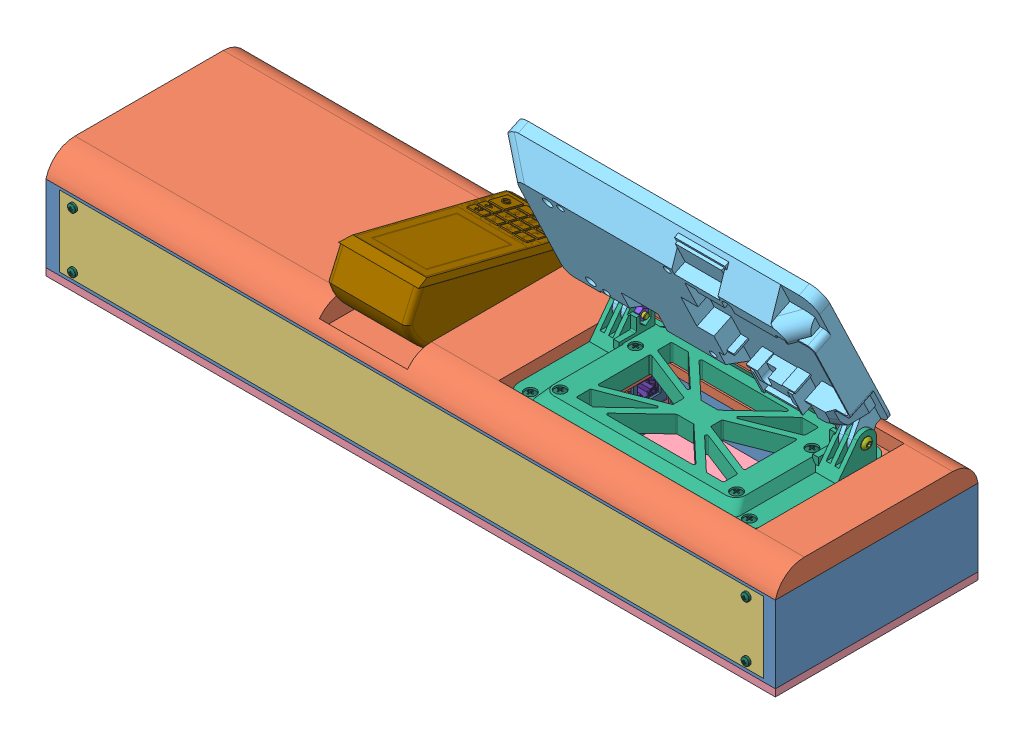
SolidWorks assembly passo4, configuration Default. Lengths in mm.
Overall size (512.8 198.81 144.85).
59 component instances, 33 part files, 93 mates.
Components (placement in the parent):
- Suporte do display correto-1: Suporte do display correto [Default] at origin size (512.8 54 142.48)
- tampa do suporte do display-2: tampa do suporte do display [Default] at (0 54 0) size (512.8 16 142.48)
- tampa de trás-2: tampa de trás [Default] at (0.9178 -87.8869 61.08) size (495 50 10)
- tampa de baixo-1: tampa de baixo [Default] at (169.3288 -5 -21.589) size (512.8 5 142.48)
- Ensamble_soporte-1: Ensamble_soporte [Predeterminado] at (197.1676 161.3746 175.3422) x (-1 0 0) z (0 0 -1) size (217.5 133.81 100.38)
  - DISPLAY-1: DISPLAY [Predeterminado] at (81.3171 -25.9151 184.231) x (1 0 0) z (0 -0.901679 0.432406) size (217.5 26.49 123.5)
  - Base-1: Base [Predeterminado] at (64.5671 -89.3746 173.3021) size (174 28.5 97.02)
  - socket button head cap screw_am-1: socket button head cap screw_am [B18.3.4M - 4 x 0.7 x 20 SBHCS --N] at (-24.6329 -80.3746 204.8021) size (22.2 7.6 7.6)
  - socket button head cap screw_am-2: socket button head cap screw_am [B18.3.4M - 4 x 0.7 x 20 SBHCS --N] at (153.7671 -80.3746 204.8021) x (-1 0 0) z (0 0.924225 0.381849) size (22.2 7.6 7.6)
  - hex nut style 2_am-2: hex nut style 2_am [B18.2.4.2M - Hex nut, Style 2,  M4 x 0.7 --D-N] at (-4.6329 -80.3746 204.8021) x (0 0 -1) z (1 0 0) size (7 8.08 3.8)
  - hex nut style 2_am-3: hex nut style 2_am [B18.2.4.2M - Hex nut, Style 2,  M4 x 0.7 --D-N] at (133.7671 -80.3746 204.8021) x (0 0 1) z (-1 0 0) size (7 8.08 3.8)
- Q80 POS Terminal Detailed-1: Q80 POS Terminal Detailed [Default] at (-35.7653 93.2106 -4.0254) x (-1 0 -0.000265) z (0.000257 -0.242857 -0.970062) size (59.7 50.26 131.44)
- Raspberry Pi 4 Model B-1: Raspberry Pi 4 Model B [Default] at (3.381 13.8908 -27.987) size (88.99 19.9 58.4)
  - PCB, RPi4ModelB-1: PCB, RPi4ModelB [Default] at origin size (85 1.6 56)
  - Broadcom BCM2711B0 CPU, RPi4ModelB-1: Broadcom BCM2711B0 CPU, RPi4ModelB [Default] at (-13.25 0.8 -4.5) size (15 2.3 15)
  - 2.54 mm DUPONT MALE PIN HEADER, POE, 2X2, RPi4ModelB-1: 2.54 mm DUPONT MALE PIN HEADER, POE, 2X2, RPi4ModelB [Default] at (19 0.8 -18.5) size (5.08 11.3 5.08)
  - 2.54 mm DUPONT MALE PIN HEADER, IO, 2X20, RPi4ModelB-1: 2.54 mm DUPONT MALE PIN HEADER, IO, 2X20, RPi4ModelB [Default] at (-10 0.8 -24.5) size (50.8 11.3 5.08)
  - Camera Connector, RPi4ModelB-1: Camera Connector, RPi4ModelB [Default] at (4 0.8 16.5) x (0 0 -1) z (1 0 0) size (22.4 5.68 5.07)
  - Microphone Plug, RPi4ModelB-1: Microphone Plug, RPi4ModelB [Default] at (11.5 0.8 21.65) size (7.23 7.55 15)
  - Display Connector, RPi4ModelB-1: Display Connector, RPi4ModelB [Default] at (-38.5 0.8 0) x (0 0 1) z (-1 0 0) size (22.4 5.68 5.07)
  - Gigabit Ethernet Port, RPi4ModelB-1: Gigabit Ethernet Port, RPi4ModelB [Default] at (45.5 7.55 -17.75) x (0 0 -1) z (1 0 0) size (16.2 17.24 21.64)
  - Female Micro HDMI Connector, RPi4ModelB-2: Female Micro HDMI Connector, RPi4ModelB [Default] at (-3 0.8 27.3875) size (6.5 3.51 7.5)
  - Female Micro HDMI Connector, RPi4ModelB-3: Female Micro HDMI Connector, RPi4ModelB [Default] at (-16.5 0.8 27.3875) size (6.5 3.51 7.5)
  - Female USB Type C Connector, RPi4ModelB-1: Female USB Type C Connector, RPi4ModelB [Default] at (-31.3 0.8 26.5419) size (8.94 3.96 7.9)
  - 2X USB3.0 PORTS, RPi4ModelB-2: 2X USB3.0 PORTS, RPi4ModelB [Default] at (37.07 0.8 1) size (17.47 19.41 15.68)
  - 91D77 D9WHV 778K, 4 GB LPDDR4 SDRAM, RPi4ModelB-1: 91D77 D9WHV 778K, 4 GB LPDDR4 SDRAM, RPi4ModelB [Default] at (2.25 0.8 -4.5) size (10 0.8 14.5)
  - Cypress CYW43455 Wireless Module Cover, RPi4ModelB-1: Cypress CYW43455 Wireless Module Cover, RPi4ModelB [Default] at (-30.5 0.8 -14.5) size (11 1.6 13)
  - SD Card Slot, RPi4ModelB-1: SD Card Slot, RPi4ModelB [Default] at (-35.3 -0.8 0) x (0 0 -1) z (-1 0 0) size (11.95 1.45 11.4)
  - VIA VL805 PCIe USB 3.0 controller, RPi4ModelB-1: VIA VL805 PCIe USB 3.0 controller, RPi4ModelB [Default] at (17.5 0.8 4) size (8.8 0.8 8.8)
  - 2X USB2.0 PORTS, RPi4ModelB-1: 2X USB2.0 PORTS, RPi4ModelB [Default] at (37.065 0.65 19) size (17.87 19.16 15.33)
  - Broadcom BCM54213PE Gigabit Ethernet Transceiver, RPi4ModelB-1: Broadcom BCM54213PE Gigabit Ethernet Transceiver, RPi4ModelB [Default] at (16.5 0.8 -10) size (6.8 1 6.8)
  - MxL7704 Universal PMIC, RPi4ModelB-1: MxL7704 Universal PMIC, RPi4ModelB [Default] at (-32.5 0.8 16) size (5.4 0.8 5.4)
- Base.step-1: Base.step [Default] at (2.881 7 -28.4) x (0 0 1) z (1 0 0) size (61 28.5 95)
- assemb parafuso-1: assemb parafuso [Default] at (21.2097 -5.2538 -61.965) x (0 -1 0) z (0 0 1) size (11.08 5.54 5)
  - M2.5 X 4.step-1: M2.5 X 4.step [Default] at (-22.0346 1.1713 9.478) size (5.07 5 5)
  - Clinching Stand off M 2.5X 61.step-2: Clinching Stand off M 2.5X 61.step [Default] at (-12.9287 1.1713 9.478) x (-1 0 0) z (0 0 1) size (6.01 5.54 4.8)
- assemb parafuso-2: assemb parafuso [Default] at (-36.7903 -5.2538 -61.965) x (0 -1 0) z (0 0 1) size (11.08 5.54 5)
  - M2.5 X 4.step-1: M2.5 X 4.step [Default] at (-22.0346 1.1713 9.478) size (5.07 5 5)
  - Clinching Stand off M 2.5X 61.step-2: Clinching Stand off M 2.5X 61.step [Default] at (-12.9287 1.1713 9.478) x (-1 0 0) z (0 0 1) size (6.01 5.54 4.8)
- assemb parafuso-3: assemb parafuso [Default] at (21.2097 -5.2538 -12.965) x (0 -1 0) z (0 0 1) size (11.08 5.54 5)
  - M2.5 X 4.step-1: M2.5 X 4.step [Default] at (-22.0346 1.1713 9.478) size (5.07 5 5)
  - Clinching Stand off M 2.5X 61.step-2: Clinching Stand off M 2.5X 61.step [Default] at (-12.9287 1.1713 9.478) x (-1 0 0) z (0 0 1) size (6.01 5.54 4.8)
- assemb parafuso-4: assemb parafuso [Default] at (-36.7903 -5.2538 -12.965) x (0 -1 0) z (0 0 1) size (11.08 5.54 5)
  - M2.5 X 4.step-1: M2.5 X 4.step [Default] at (-22.0346 1.1713 9.478) size (5.07 5 5)
  - Clinching Stand off M 2.5X 61.step-2: Clinching Stand off M 2.5X 61.step [Default] at (-12.9287 1.1713 9.478) x (-1 0 0) z (0 0 1) size (6.01 5.54 4.8)
- Cover.step-2: Cover.step [Default] at (1.881 35.5 -28.9) x (0 0 1) z (-1 0 0) size (65 37 97)
- Microcontrolador MSP430G2-2: Microcontrolador MSP430G2 [Predeterminado] at (-150.1159 2 -54.4475) x (0 0 -1) z (1 0 0) size (51 9 66)
- pan cross head_am-1: pan cross head_am [B18.6.7M - M4 x 0.7 x 8 Type I Cross Recessed PHMS --8N] at (209.6005 66.1 42.54) x (0 -1 0) z (0 0 1) size (11.07 8 8)
- pan cross head_am-2: pan cross head_am [B18.6.7M - M4 x 0.7 x 8 Type I Cross Recessed PHMS --8N] at (194.6005 72.1 36.54) x (0 -1 0) z (0 0 1) size (11.07 8 8)
- pan cross head_am-3: pan cross head_am [B18.6.7M - M4 x 0.7 x 8 Type I Cross Recessed PHMS --8N] at (194.6005 72.1 -16.46) x (0 -1 0) z (0 0 1) size (11.07 8 8)
- pan cross head_am-4: pan cross head_am [B18.6.7M - M4 x 0.7 x 8 Type I Cross Recessed PHMS --8N] at (70.6005 72.1 -16.46) x (0 -1 0) z (0 0 1) size (11.07 8 8)
- pan cross head_am-5: pan cross head_am [B18.6.7M - M4 x 0.7 x 8 Type I Cross Recessed PHMS --8N] at (70.6005 72.1 36.54) x (0 -1 0) z (0 0 1) size (11.07 8 8)
- pan cross head_am-6: pan cross head_am [B18.6.7M - M4 x 0.7 x 8 Type I Cross Recessed PHMS --8N] at (55.6005 66.1 42.54) x (0 -1 0) z (0 0 1) size (11.07 8 8)
- pan cross head_am-7: pan cross head_am [B18.6.7M - M4 x 0.7 x 8 Type I Cross Recessed PHMS --8N] at (209.6005 66.1 -38.46) x (0 -1 0) z (0 0 1) size (11.07 8 8)
- pan cross head_am-8: pan cross head_am [B18.6.7M - M4 x 0.7 x 8 Type I Cross Recessed PHMS --8N] at (55.6005 66.1 -38.46) x (0 -1 0) z (0 0 1) size (11.07 8 8)
- pan cross head_am-9: pan cross head_am [B18.6.7M - M3 x 0.5 x 16 Type I Cross Recessed PHMS --16N] at (236.5887 46.5861 73.48) x (0 0 -1) z (1 0 0) size (18.37 5.6 5.6)
- pan cross head_am-10: pan cross head_am [B18.6.7M - M3 x 0.5 x 16 Type I Cross Recessed PHMS --16N] at (236.5887 7.345 73.48) x (0 0 -1) z (1 0 0) size (18.37 5.6 5.6)
- pan cross head_am-11: pan cross head_am [B18.6.7M - M3 x 0.5 x 16 Type I Cross Recessed PHMS --16N] at (-237.0024 46.5861 73.48) x (0 0 -1) z (1 0 0) size (18.37 5.6 5.6)
- pan cross head_am-12: pan cross head_am [B18.6.7M - M3 x 0.5 x 16 Type I Cross Recessed PHMS --16N] at (-237.0024 7.345 73.48) x (0 0 -1) z (1 0 0) size (18.37 5.6 5.6)
Mates (geometry in assembly coordinates):
- Coincident1: coincident anti-aligned: plane of Suporte do display correto-1 through (0 54 0) normal (0 1 0); plane of tampa do suporte do display-2 through (0 54 0) normal (0 -1 0)
- Coincident2: coincident aligned: plane of Suporte do display correto-1 through (-256.4 54 -71.4) normal (0 0 -1); plane of tampa do suporte do display-2 through (-256.4 70 -71.4) normal (0 0 -1)
- Coincident3: coincident aligned: plane of Suporte do display correto-1 through (256.4 54 -71.4) normal (1 0 0); plane of tampa do suporte do display-2 through (256.4 70 -71.4) normal (1 0 0)
- Coincident5: coincident anti-aligned: plane of Suporte do display correto-1 through (0 0 61.08) normal (0 0 1); plane of tampa de trás-2 through (0.9178 -87.8869 61.08) normal (0 0 -1)
- Coincident6: coincident anti-aligned: plane of Suporte do display correto-1 through (248.0677 52.1414 61.08) normal (-1 0 0); plane of tampa de trás-2 through (248.0677 52.1414 71.08) normal (1 0 0)
- Coincident7: coincident anti-aligned: plane of Suporte do display correto-1 through (-246.9323 2.1414 61.08) normal (0 1 0); plane of tampa de trás-2 through (-246.9323 2.1414 71.08) normal (0 -1 0)
- Coincident8: coincident anti-aligned: plane of Suporte do display correto-1 through (0 0 0) normal (0 -1 0); plane of tampa de baixo-1 through (169.3288 0 -21.589) normal (0 1 0)
- Coincident9: coincident aligned: plane of Suporte do display correto-1 through (-256.4 54 -71.4) normal (-1 0 0); plane of tampa de baixo-1 through (-256.4 0 -71.4) normal (-1 0 0)
- Coincident10: coincident aligned: plane of tampa de trás-2 through (0.9178 -87.8869 71.08) normal (0 0 1); plane of tampa de baixo-1 through (-256.4 0 71.08) normal (0 0 1)
- Coincident11: coincident anti-aligned: plane of tampa do suporte do display-2 through (0 60 0) normal (0 1 0); plane of Ensamble_soporte-1/Base-1 through (209.6005 60 -36.46) normal (0 -1 0)
- Coincident13: coincident anti-aligned: plane of tampa do suporte do display-2 through (41.49 60 50.54) normal (0 0 -1); plane of Ensamble_soporte-1/Base-1 through (209.6005 66 50.54) normal (0 0 1)
- Coincident15: coincident anti-aligned: plane of Ensamble_soporte-1/Base-1 through (194.6005 69 36.54) normal (0 1 0); plane of Parafuso Sextavado M10-2 through (196.9099 69 40.54) normal (0 -1 0)
- Tangent1: tangent aligned: cylinder of Ensamble_soporte-1/Base-1 through (194.6005 69 36.54) axis (0 1 0) radius 4; plane of Parafuso Sextavado M10-2 through (192.2911 75.4 40.54) normal (0 0 1)
- Tangent2: tangent aligned: cylinder of Ensamble_soporte-1/Base-1 through (194.6005 69 36.54) axis (0 1 0) radius 4; plane of Parafuso Sextavado M10-2 through (196.9099 75.4 40.54) normal (0.866025 0 0.5)
- Coincident17: coincident anti-aligned: plane of Ensamble_soporte-1/Base-1 through (70.6005 69 36.54) normal (0 1 0); plane of Parafuso Sextavado M10-4 through (74.6005 69 34.2306) normal (0 -1 0)
- Tangent3: tangent aligned: cylinder of Ensamble_soporte-1/Base-1 through (70.6005 69 36.54) axis (0 1 0) radius 4; plane of Parafuso Sextavado M10-4 through (66.6005 75.4 34.2306) normal (-1 0 0)
- Tangent4: tangent aligned: cylinder of Ensamble_soporte-1/Base-1 through (70.6005 69 36.54) axis (0 1 0) radius 4; plane of Parafuso Sextavado M10-4 through (74.6005 75.4 34.2306) normal (0.5 0 -0.866025)
- Coincident18: coincident anti-aligned: plane of Ensamble_soporte-1/Base-1 through (55.6005 63 42.54) normal (0 1 0); plane of Parafuso Sextavado M10-5 through (59.6005 63 39.8752) normal (0 -1 0)
- Tangent6: tangent aligned: cylinder of Ensamble_soporte-1/Base-1 through (55.6005 63 42.54) axis (0 1 0) radius 4; plane of Parafuso Sextavado M10-5 through (59.6005 69.4 44.494) normal (1 0 0)
- Lock1: lock: unknown of tampa do suporte do display-2; unknown of Parafuso Sextavado M10-5
- Coincident19: coincident anti-aligned: plane of Ensamble_soporte-1/Base-1 through (209.6005 63 42.54) normal (0 1 0); plane of Parafuso Sextavado M10-6 through (213.7574 63 40.9265) normal (0 -1 0)
- Tangent9: tangent aligned: cylinder of Ensamble_soporte-1/Base-1 through (209.6005 63 42.54) axis (0 1 0) radius 4; plane of Parafuso Sextavado M10-6 through (208.7461 69.4 47.1625) normal (0.361863 0 0.932231)
- Lock2: lock: unknown of tampa do suporte do display-2; unknown of Parafuso Sextavado M10-6
- Concentric3: concentric anti-aligned: cylinder of Base.step-1 through (-34.619 7 -52.9) axis (0 1 0) radius 2; cylinder of Rubber Grommet.step-1 through (-150.9859 -46.5621 -148.5283) axis (0 -1 0) radius 1.75
- Concentric4: concentric anti-aligned: cylinder of Base.step-1 through (-34.619 7 -3.9) axis (0 1 0) radius 2; cylinder of Rubber Grommet.step-2 through (-150.9859 -46.5088 -99.5283) axis (0 -1 0) radius 1.75
- Concentric5: concentric anti-aligned: circle of Base.step-1; circle of Rubber Grommet.step-3
- Concentric6: concentric anti-aligned: circle of Base.step-1; circle of Rubber Grommet.step-4
- Coincident24: coincident anti-aligned: plane of Raspberry Pi 4 Model B-1/Gigabit Ethernet Port, RPi4ModelB-1 through (48.881 21.4408 -45.737) normal (1 0 0); plane of Base.step-1 through (48.881 7 -28.4) normal (-1 0 0)
- Concentric8: concentric aligned: cylinder of Raspberry Pi 4 Model B-1/PCB, RPi4ModelB-1 through (22.381 14.6908 -52.487) axis (0 1 0) radius 1.35; cylinder of assemb parafuso-1/M2.5 X 4.step-1 through (22.381 42.1808 -52.487) axis (0 1 0) radius 1.25
- Coincident27: coincident anti-aligned: plane of Raspberry Pi 4 Model B-1/PCB, RPi4ModelB-1 through (22.381 14.6808 -52.487) normal (0 1 0); plane of assemb parafuso-1/M2.5 X 4.step-1 through (23.631 14.6808 -52.487) normal (0 -1 0)
- Concentric9: concentric aligned: cylinder of Raspberry Pi 4 Model B-1/PCB, RPi4ModelB-1 through (-35.619 14.6908 -52.487) axis (0 1 0) radius 1.35; cylinder of assemb parafuso-2/M2.5 X 4.step-1 through (-35.619 42.1808 -52.487) axis (0 1 0) radius 1.25
- Coincident28: coincident anti-aligned: plane of Raspberry Pi 4 Model B-1/PCB, RPi4ModelB-1 through (-35.619 14.6808 -52.487) normal (0 1 0); plane of assemb parafuso-2/M2.5 X 4.step-1 through (-34.369 14.6808 -52.487) normal (0 -1 0)
- Lock3: lock: unknown of Raspberry Pi 4 Model B-1/PCB, RPi4ModelB-1; unknown of assemb parafuso-2/M2.5 X 4.step-1
- Lock4: lock: unknown of Raspberry Pi 4 Model B-1/PCB, RPi4ModelB-1; unknown of assemb parafuso-1/M2.5 X 4.step-1
- Lock5: lock: unknown of Base.step-1; unknown of assemb parafuso-1/Clinching Stand off M 2.5X 61.step-2
- Lock6: lock: unknown of Base.step-1; unknown of assemb parafuso-1/Clinching Stand off M 2.5X 61.step-2
- Concentric15: concentric aligned: cylinder of Raspberry Pi 4 Model B-1/PCB, RPi4ModelB-1 through (22.381 14.6908 -3.487) axis (0 1 0) radius 1.35; cylinder of assemb parafuso-3/M2.5 X 4.step-1 through (22.381 42.1808 -3.487) axis (0 1 0) radius 1.25
- Coincident30: coincident anti-aligned: plane of Raspberry Pi 4 Model B-1/PCB, RPi4ModelB-1 through (22.381 14.6808 -3.487) normal (0 1 0); plane of assemb parafuso-3/M2.5 X 4.step-1 through (23.631 14.6808 -3.487) normal (0 -1 0)
- Lock8: lock: unknown of Raspberry Pi 4 Model B-1/PCB, RPi4ModelB-1; unknown of assemb parafuso-3/M2.5 X 4.step-1
- Concentric16: concentric aligned: cylinder of Raspberry Pi 4 Model B-1/PCB, RPi4ModelB-1 through (-35.619 14.6908 -3.487) axis (0 1 0) radius 1.35; cylinder of assemb parafuso-4/M2.5 X 4.step-1 through (-35.619 42.1808 -3.487) axis (0 1 0) radius 1.25
- Coincident33: coincident anti-aligned: plane of Raspberry Pi 4 Model B-1/PCB, RPi4ModelB-1 through (-35.619 14.6808 -3.487) normal (0 1 0); plane of assemb parafuso-4/M2.5 X 4.step-1 through (-34.369 14.6808 -3.487) normal (0 -1 0)
- Lock10: lock: unknown of Raspberry Pi 4 Model B-1/PCB, RPi4ModelB-1; unknown of assemb parafuso-4/M2.5 X 4.step-1
- Coincident41: coincident anti-aligned: plane of Base.step-1 through (50.381 35.5 -58.9) normal (0 1 0); plane of Cover.step-2 through (1.881 35.5 -28.9) normal (0 -1 0)
- Coincident42: coincident anti-aligned: plane of Base.step-1 through (50.381 35.5 2.1) normal (0 0 1); plane of Cover.step-2 through (1.881 35.5 2.1) normal (0 0 -1)
- Coincident43: coincident anti-aligned: plane of tampa de baixo-1 through (169.3288 0 -21.589) normal (0 1 0); plane of Cover.step-2 through (1.881 0 -28.9) normal (0 -1 0)
- Coincident44: coincident aligned: plane of Base.step-1 through (50.381 7 -28.4) normal (1 0 0); plane of Cover.step-2 through (50.381 37 -61.4) normal (1 0 0)
- Coincident45: coincident anti-aligned: plane of Suporte do display correto-1 through (0 54 -61.4) normal (0 0 1); plane of Cover.step-2 through (1.881 35.5 -61.4) normal (0 0 -1)
- Coincident46: coincident anti-aligned: plane of Suporte do display correto-1 through (50.381 0 8.6) normal (-1 0 0); plane of Cover.step-2 through (50.381 0 2.1) normal (1 0 0)
- Coincident48: coincident anti-aligned: plane of Suporte do display correto-1 through (-62.0917 2 -61.4) normal (0 1 0); plane of Microcontrolador MSP430G2-2 through (-150.1159 2 -54.4475) normal (0 -1 0)
- Coincident49: coincident anti-aligned: plane of Suporte do display correto-1 through (0 54 -61.4) normal (0 0 1); plane of Microcontrolador MSP430G2-2 through (-179.1309 3 -61.4) normal (0 0 -1)
- Coincident50: coincident anti-aligned: plane of Suporte do display correto-1 through (-179.1309 0 -68.4711) normal (1 0 0); plane of Microcontrolador MSP430G2-2 through (-179.1309 3 -10.4) normal (-1 0 0)
- Concentric18: concentric aligned: cylinder of Ensamble_soporte-1/Base-1 through (209.6005 63 42.54) axis (0 1 0) radius 4; cylinder of pan cross head_am-1 through (209.6005 91.5 42.54) axis (0 1 0) radius 4
- Coincident52: coincident anti-aligned: plane of Ensamble_soporte-1/Base-1 through (209.6005 63 42.54) normal (0 1 0); plane of pan cross head_am-1 through (211.6005 63 42.54) normal (0 -1 0)
- Concentric19: concentric aligned: cylinder of Ensamble_soporte-1/Base-1 through (194.6005 59.999 36.54) axis (0 1 0) radius 2; cylinder of pan cross head_am-2 through (194.6005 97.5 36.54) axis (0 1 0) radius 4
- Coincident53: coincident anti-aligned: plane of Ensamble_soporte-1/Base-1 through (194.6005 69 36.54) normal (0 1 0); plane of pan cross head_am-2 through (196.6005 69 36.54) normal (0 -1 0)
- Concentric20: concentric aligned: cylinder of Ensamble_soporte-1/Base-1 through (194.6005 59.999 -16.46) axis (0 1 0) radius 2; cylinder of pan cross head_am-3 through (194.6005 97.5 -16.46) axis (0 1 0) radius 4
- Coincident54: coincident anti-aligned: plane of Ensamble_soporte-1/Base-1 through (194.6005 69 -16.46) normal (0 1 0); plane of pan cross head_am-3 through (196.6005 69 -16.46) normal (0 -1 0)
- Concentric21: concentric aligned: cylinder of Ensamble_soporte-1/Base-1 through (70.6005 59.999 -16.46) axis (0 1 0) radius 2; cylinder of pan cross head_am-4 through (70.6005 97.5 -16.46) axis (0 1 0) radius 4
- Coincident55: coincident anti-aligned: plane of Ensamble_soporte-1/Base-1 through (70.6005 69 -16.46) normal (0 1 0); plane of pan cross head_am-4 through (72.6005 69 -16.46) normal (0 -1 0)
- Concentric22: concentric aligned: cylinder of Ensamble_soporte-1/Base-1 through (70.6005 59.999 36.54) axis (0 1 0) radius 2; cylinder of pan cross head_am-5 through (70.6005 97.5 36.54) axis (0 1 0) radius 4
- Coincident56: coincident anti-aligned: plane of Ensamble_soporte-1/Base-1 through (70.6005 69 36.54) normal (0 1 0); plane of pan cross head_am-5 through (72.6005 69 36.54) normal (0 -1 0)
- Concentric23: concentric aligned: cylinder of Ensamble_soporte-1/Base-1 through (55.6005 63 42.54) axis (0 1 0) radius 4; cylinder of pan cross head_am-6 through (55.6005 91.5 42.54) axis (0 1 0) radius 4
- Coincident57: coincident anti-aligned: plane of Ensamble_soporte-1/Base-1 through (55.6005 63 42.54) normal (0 1 0); plane of pan cross head_am-6 through (57.6005 63 42.54) normal (0 -1 0)
- Concentric24: concentric aligned: cylinder of Ensamble_soporte-1/Base-1 through (209.6005 63 -38.46) axis (0 1 0) radius 4; cylinder of pan cross head_am-7 through (209.6005 91.5 -38.46) axis (0 1 0) radius 4
- Coincident58: coincident anti-aligned: plane of Ensamble_soporte-1/Base-1 through (209.6005 63 -38.46) normal (0 1 0); plane of pan cross head_am-7 through (211.6005 63 -38.46) normal (0 -1 0)
- Concentric25: concentric aligned: cylinder of Ensamble_soporte-1/Base-1 through (55.6005 63 -38.46) axis (0 1 0) radius 4; cylinder of pan cross head_am-8 through (55.6005 91.5 -38.46) axis (0 1 0) radius 4
- Coincident59: coincident anti-aligned: plane of Ensamble_soporte-1/Base-1 through (55.6005 63 -38.46) normal (0 1 0); plane of pan cross head_am-8 through (57.6005 63 -38.46) normal (0 -1 0)
- Coincident60: coincident anti-aligned: plane of tampa do suporte do display-2 through (0 55 0) normal (0 1 0); plane of Q80 POS Terminal Detailed-1 through (-58.5258 55 35.8413) normal (0 -1 0)
- Concentric26: concentric aligned: cylinder of tampa de trás-2 through (236.5887 46.5861 51.08) axis (0 0 1) radius 1.5; cylinder of hex flange machine screw_am-1 through (236.5887 46.5861 99.68) axis (0 0 1) radius 1.5
- Coincident61: coincident anti-aligned: plane of tampa de trás-2 through (0.9178 -87.8869 71.08) normal (0 0 1); plane of hex flange machine screw_am-1 through (236.5887 48.0861 71.08) normal (0 0 -1)
- Concentric27: concentric aligned: cylinder of tampa de trás-2 through (236.5887 7.345 51.08) axis (0 0 1) radius 1.5; cylinder of hex flange machine screw_am-2 through (236.5887 7.345 99.68) axis (0 0 1) radius 1.5
- Coincident62: coincident anti-aligned: plane of tampa de trás-2 through (0.9178 -87.8869 71.08) normal (0 0 1); plane of hex flange machine screw_am-2 through (236.5887 8.845 71.08) normal (0 0 -1)
- Concentric28: concentric aligned: cylinder of tampa de trás-2 through (-237.0024 46.5861 51.08) axis (0 0 1) radius 1.5; cylinder of hex flange machine screw_am-3 through (-237.0024 46.5861 99.68) axis (0 0 1) radius 1.5
- Coincident63: coincident anti-aligned: plane of tampa de trás-2 through (0.9178 -87.8869 71.08) normal (0 0 1); plane of hex flange machine screw_am-3 through (-237.0024 48.0861 71.08) normal (0 0 -1)
- Concentric29: concentric aligned: cylinder of tampa de trás-2 through (-237.0024 7.345 51.08) axis (0 0 1) radius 1.5; cylinder of hex flange machine screw_am-4 through (-237.0024 7.345 99.68) axis (0 0 1) radius 1.5
- Coincident64: coincident anti-aligned: plane of tampa de trás-2 through (0.9178 -87.8869 71.08) normal (0 0 1); plane of hex flange machine screw_am-4 through (-237.0024 8.845 71.08) normal (0 0 -1)
- Concentric30: concentric aligned: cylinder of tampa de trás-2 through (236.5887 46.5861 51.08) axis (0 0 1) radius 1.5; cylinder of pan slot head_am-1 through (236.5887 46.5861 102.4035) axis (0 0 1) radius 2.8
- Concentric31: concentric aligned: cylinder of tampa de trás-2 through (236.5887 7.345 51.08) axis (0 0 1) radius 1.5; cylinder of pan slot head_am-2 through (236.5887 7.345 98.88) axis (0 0 1) radius 2.8
- Coincident65: coincident anti-aligned: plane of tampa de trás-2 through (0.9178 -87.8869 71.08) normal (0 0 1); plane of pan slot head_am-2 through (236.5887 8.845 71.08) normal (0 0 -1)
- Concentric32: concentric aligned: cylinder of tampa de trás-2 through (-237.0024 46.5861 51.08) axis (0 0 1) radius 1.5; cylinder of pan slot head_am-3 through (-237.0024 46.5861 98.88) axis (0 0 1) radius 2.8
- Coincident66: coincident anti-aligned: plane of tampa de trás-2 through (0.9178 -87.8869 71.08) normal (0 0 1); plane of pan slot head_am-3 through (-237.0024 48.0861 71.08) normal (0 0 -1)
- Concentric33: concentric aligned: cylinder of tampa de trás-2 through (-237.0024 7.345 51.08) axis (0 0 1) radius 1.5; cylinder of pan slot head_am-4 through (-237.0024 7.345 98.88) axis (0 0 1) radius 2.8
- Coincident67: coincident anti-aligned: plane of tampa de trás-2 through (0.9178 -87.8869 71.08) normal (0 0 1); plane of pan slot head_am-4 through (-237.0024 8.845 71.08) normal (0 0 -1)
- Concentric34: concentric aligned: cylinder of tampa de trás-2 through (236.5887 46.5861 51.08) axis (0 0 1) radius 1.5; cylinder of pan slot head_am-5 through (236.5887 46.5861 98.88) axis (0 0 1) radius 2.8
- Coincident68: coincident anti-aligned: plane of tampa de trás-2 through (0.9178 -87.8869 71.08) normal (0 0 1); plane of pan slot head_am-5 through (236.5887 48.0861 71.08) normal (0 0 -1)
- Concentric35: concentric aligned: cylinder of tampa de trás-2 through (236.5887 46.5861 51.08) axis (0 0 1) radius 1.5; cylinder of pan cross head_am-9 through (236.5887 46.5861 98.88) axis (0 0 1) radius 2.8
- Coincident69: coincident anti-aligned: plane of tampa de trás-2 through (0.9178 -87.8869 71.08) normal (0 0 1); plane of pan cross head_am-9 through (236.5887 48.0861 71.08) normal (0 0 -1)
- Concentric36: concentric aligned: cylinder of tampa de trás-2 through (236.5887 7.345 51.08) axis (0 0 1) radius 1.5; cylinder of pan cross head_am-10 through (236.5887 7.345 98.88) axis (0 0 1) radius 2.8
- Coincident70: coincident anti-aligned: plane of tampa de trás-2 through (0.9178 -87.8869 71.08) normal (0 0 1); plane of pan cross head_am-10 through (236.5887 8.845 71.08) normal (0 0 -1)
- Concentric37: concentric aligned: cylinder of tampa de trás-2 through (-237.0024 46.5861 51.08) axis (0 0 1) radius 1.5; cylinder of pan cross head_am-11 through (-237.0024 46.5861 98.88) axis (0 0 1) radius 2.8
- Coincident71: coincident anti-aligned: plane of tampa de trás-2 through (0.9178 -87.8869 71.08) normal (0 0 1); plane of pan cross head_am-11 through (-237.0024 48.0861 71.08) normal (0 0 -1)
- Concentric38: concentric aligned: cylinder of tampa de trás-2 through (-237.0024 7.345 51.08) axis (0 0 1) radius 1.5; cylinder of pan cross head_am-12 through (-237.0024 7.345 98.88) axis (0 0 1) radius 2.8
- Coincident72: coincident anti-aligned: plane of tampa de trás-2 through (0.9178 -87.8869 71.08) normal (0 0 1); plane of pan cross head_am-12 through (-237.0024 8.845 71.08) normal (0 0 -1)
